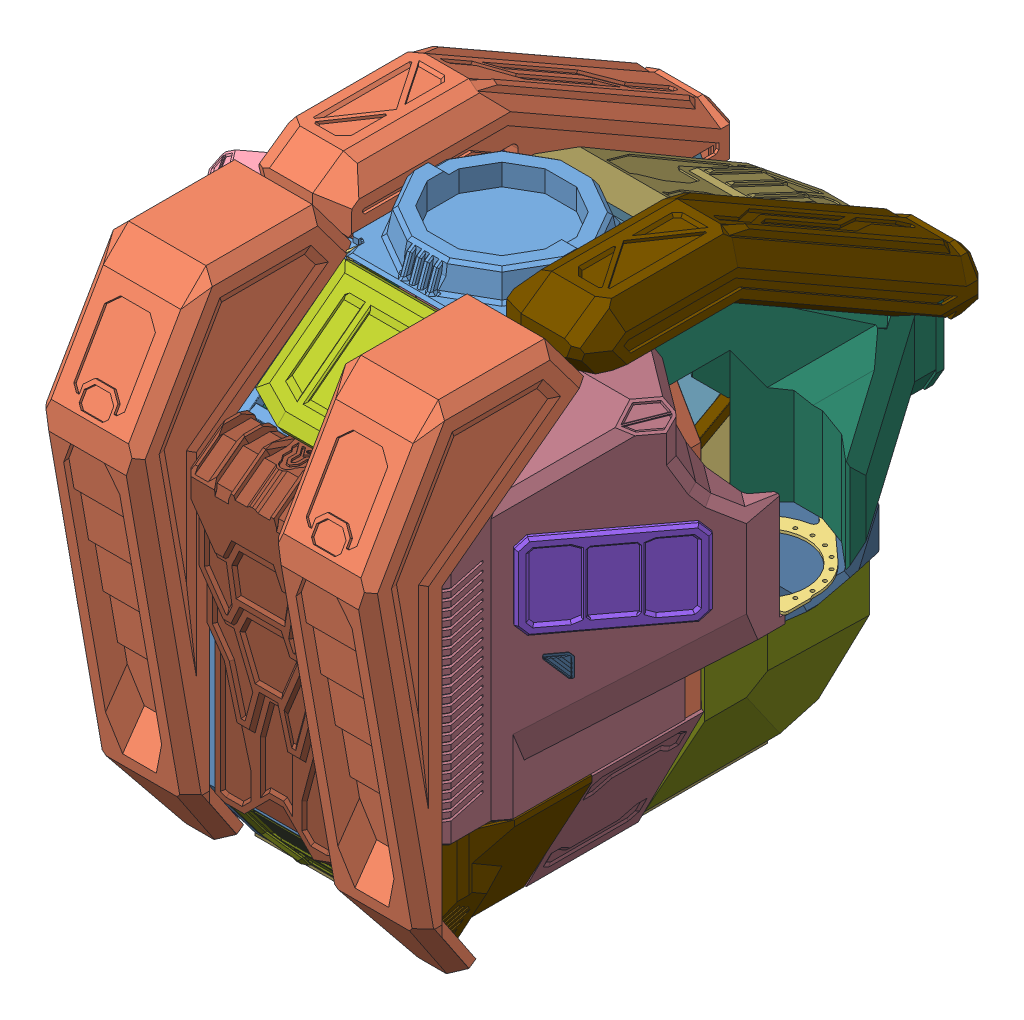
SolidWorks assembly cockpite superficie, configuration Défaut. Lengths in mm.
Overall size (2088.81 2085.24 2703.64).
117 component instances, 75 part files, 251 mates.
Components (placement in the parent):
- cockpit_segmentLAT_0-1: cockpit_segmentLAT_0 [Défaut] at origin size (80 1780 1700)
- cockpit_segmentLAT_0-2: cockpit_segmentLAT_0 [Défaut] at (-580 0 0) size (80 1780 1700)
- cockpit_segmentFACE_0-1: cockpit_segmentFACE_0 [Défaut] at (-250 0 -10.6226) size (1180 1780 80)
- Manikin_sit-1: Manikin_sit [Default] at (-178.4008 -3076.5165 -521.6706) x (-0.998263 -0.006408 -0.058563) z (0.055728 0.219684 -0.973978) size (878.99 1461.66 750.53)
  - Hips-1: Hips [Default] at (41.9716 15.4252 492.0452) x (0.998799 0.006411 -0.048571) z (0.047333 0.129538 0.990444) size (295.24 313.39 270.97)
  - Torso-1: Torso [Default] at (-29.1895 18.5281 -268.9557) x (0.995716 0.002037 -0.092438) z (0.092349 -0.071067 0.993187) size (460.89 555.97 263.41)
  - Head-2: Head [Default] at (-35.3994 3.8201 -64.7195) x (0.99996 -0.00842 0.002952) z (-0.003142 -0.022585 0.99974) size (157.49 285.21 225.45)
  - ArmLeftUpper-1: ArmLeftUpper [Default] at (-1722.5354 534.7955 -622.021) x (0.903661 -0.428241 0.002425) z (-0.067425 -0.136682 0.988318) size (245.85 241.52 164.39)
  - LegLeftUpper-1: LegLeftUpper [Default] at (-298.9777 2948.9846 3668.472) x (0.995737 -0.057217 0.072354) z (0.044237 0.984495 0.169742) size (217.98 507.99 239.38)
  - ArmLeftFore-1: ArmLeftFore [Default] at (-2325.1537 1043.3966 992.7578) x (0.576966 -0.135199 0.8055) z (-0.537701 0.679474 0.499192) size (231.54 177.84 142.38)
  - ArmLeftHand-1: ArmLeftHand [Default] at (-1973.6621 823.2165 1249.8034) x (0.681315 -0.092916 0.72607) z (-0.527105 0.625983 0.574722) size (149.66 182.81 147.58)
  - LegLeftLower-1: LegLeftLower [Default] at (-393.4208 426.2264 1183.139) x (0.993791 -0.108531 0.024512) z (0.002157 0.239057 0.971003) size (171.81 443.68 193.78)
  - LegLeftFoot-1: LegLeftFoot [Default] at (-391.5322 345.3545 592.5292) x (0.993832 -0.110241 0.012061) z (-0.008622 0.031619 0.999463) size (154.71 147.12 252.53)
  - ArmRightUpper-1: ArmRightUpper [Default] at (2412.2824 931.5079 323.6395) x (0.78978 0.59507 0.148794) z (-0.156135 -0.039556 0.986943) size (246.03 241.06 163.63)
  - ArmRightFore-1: ArmRightFore [Default] at (2450.4069 1513.5578 1822.4726) x (0.754277 0.265812 -0.600342) z (0.232424 0.747064 0.622796) size (231.51 177.54 142.76)
  - ArmRightHand-1: ArmRightHand [Default] at (726.3463 519.61 2107.5247) x (0.731421 -0.279768 -0.621895) z (0.656431 0.535891 0.530961) size (149.56 182.72 147.2)
  - LegRightUpper-1: LegRightUpper [Default] at (121.5915 3105.6896 3713.3645) x (0.987695 0.156074 -0.009999) z (-0.153555 0.97991 0.127269) size (216.84 507.94 244.77)
  - LegRightLower-1: LegRightLower [Default] at (672.1591 446.131 902.2036) x (0.976643 0.210274 0.044195) z (-0.073882 0.135492 0.98802) size (171.15 451.19 193.59)
  - LegRightFoot-1: LegRightFoot [Default] at (695.8533 419.9505 536.4877) x (0.976144 0.210831 0.051905) z (-0.054843 0.008108 0.998462) size (155.81 152.18 252.53)
- cockpit_segment_40x40_0-1: cockpit_segment_40x40_0 [Défaut] at (80 1283.2129 -10) size (258 40 730)
- cockpit_segment_40x40_0-2: cockpit_segment_40x40_0 [Défaut] at (-580 1323.2129 -10) x (-1 0 0) z (0 0 1) size (258 40 730)
- cockpit_segment_40x40_0-3: cockpit_segment_40x40_0 [Défaut] at (80 960 -10) size (258 40 730)
- cockpit_segment_40x40_0-4: cockpit_segment_40x40_0 [Défaut] at (-580 1000 -10) x (-1 0 0) z (0 0 1) size (258 40 730)
- cockpit_segmentFACE_0-2: cockpit_segmentFACE_0 [Défaut] at (-250 0 333.3333) size (1180 1780 80)
- cockpit_poutre40x80x500-5: cockpit_poutre40x80x500 [Défaut] at (-500 250 920) x (0 1 0) z (1 0 0) size (80 40 500)
- cockpit_poutre40x80x500-6: cockpit_poutre40x80x500 [Défaut] at (0 1330 920) x (0 -1 0) z (-1 0 0) size (80 40 500)
- cockpit_poutre40x80x500-7: cockpit_poutre40x80x500 [Défaut] at (-500 -40 -436.5685) x (0 0 -1) z (1 0 0) size (80 40 500)
- cockpit_poutre40x40x366-1: cockpit_poutre40x40x366 [Défaut] at (-840 1270.6802 69.3333) size (40 40 264)
- cockpit_poutre40x40x366-2: cockpit_poutre40x40x366 [Défaut] at (-840 440.3702 69.3333) size (40 40 264)
- cockpit_poutre40x40x366-3: cockpit_poutre40x40x366 [Défaut] at (300 1270.6802 69.3774) size (40 40 264)
- cockpit_poutre40x40x366-4: cockpit_poutre40x40x366 [Défaut] at (300 440.3702 69.3774) size (40 40 264)
- cockpit_poutre40x40x366-5: cockpit_poutre40x40x366 [Défaut] at (-840 960 67.3333) size (40 40 264)
- cockpit_poutre40x40x366-6: cockpit_poutre40x40x366 [Défaut] at (300 960 69.3774) size (40 40 264)
- bras_fixation_1-1: bras_fixation_1 [Défaut] at (340 990 512.9113) size (615.49 10 1037.05)
- bras_fixation_1-2: bras_fixation_1 [Défaut] at (-840 1000 512.9113) x (-1 0 0) z (0 0 1) size (615.49 10 1037.05)
- cockpit_poutre40x80x500-8: cockpit_poutre40x80x500 [Défaut] at (-500 396.2581 380) x (0 1 0) z (1 0 0) size (80 40 500)
- traverse_pente1-1: traverse_pente1 [Défaut] at (338 209.1038 -10.6226) x (-1 0 0) z (0 0 -1) size (257.78 292.58 728.37)
- traverse_pente1_sym-1: traverse_pente1_sym [Défaut] at (-838 209.1038 -10.6226) size (257.78 292.58 733.7)
- cockpit_poutre40x80x500-9: cockpit_poutre40x80x500 [Défaut] at (0 1340.3258 816.6212) x (0 0.90883 0.417168) z (-1 0 0) size (80 40 500)
- cockpit_segment_40x40_1_soutien_bras-1: cockpit_segment_40x40_1_soutien_bras [Défaut] at (-840 990 69.3774) x (0 -1 0) z (1 0 0) size (350 80 400)
- cockpit_segment_40x40_1_soutien_bras-2: cockpit_segment_40x40_1_soutien_bras [Défaut] at (340 990 -10.6226) x (0 -1 0) z (-1 0 0) size (350 80 400)
- cockpit_segment_40x40_2_back-1: cockpit_segment_40x40_2_back [Défaut] at (80 1310.6802 413.3333) x (1 0 0) z (0 0 -1) size (260 40 546)
- cockpit_segment_40x40_2_back-2: cockpit_segment_40x40_2_back [Défaut] at (-580 1270.6802 413.3333) x (-1 0 0) z (0 0 -1) size (260 40 546)
- attache_porte-1: attache_porte [Défaut] at (-500 1641.4369 -183.108) x (0 0.496139 0.868243) z (-1 0 0) size (198.66 73.18 10)
- attache_porte-2: attache_porte [Défaut] at (80 1641.4369 -183.108) x (0 0.496139 0.868243) z (-1 0 0) size (198.66 73.18 10)
- attache_porte-3: attache_porte [Défaut] at (-570 1641.4369 -183.108) x (0 0.496139 0.868243) z (-1 0 0) size (198.66 73.18 10)
- attache_porte-4: attache_porte [Défaut] at (10 1641.4369 -183.108) x (0 0.496139 0.868243) z (-1 0 0) size (198.66 73.18 10)
- axeO20.25_700-1: axeO20.25_700 [Défaut] at (-600 1702.1061 -146.8375) x (0 0.072457 -0.997372) z (1 0 0) size (20 20 700)
- Capot-1: Capot [Défaut] at (-480 1702.1061 -146.8375) x (-1 0 0) z (0 -0.505329 -0.862927) size (560 946.97 1454.08)
  - Capot1-1: Capot1 [Défaut] at origin size (10 749.16 1208.3)
  - Capot1-2: Capot1 [Défaut] at (-470 0 0) size (10 749.16 1208.3)
  - cockpit_poutre40x40x480-1: cockpit_poutre40x40x480 [Défaut] at (10 -20 40) x (0 0 1) z (-1 0 0) size (40 40 480)
  - cockpit_poutre40x40x480-2: cockpit_poutre40x40x480 [Défaut] at (10 -32.3205 751.7543) x (0 0.866025 0.5) z (-1 0 0) size (40 40 480)
  - cockpit_poutre40x40x480-3: cockpit_poutre40x40x480 [Défaut] at (10 -683.1793 1118.6603) x (0 -0.866025 0.5) z (-1 0 0) size (40 40 480)
  - Capot2-1: Capot2 [Défaut] at (-230 -26.9447 40) x (-1 0 0) z (0 0 -1) size (560 161.69 1100)
  - Capot3-1: Capot3 [Défaut] at (20 -892.9701 1297.518) x (-1 0 0) z (0 -0.5 -0.866025) size (500 906.77 276.51)
  - Capot4-1: Capot4 [Défaut] at (-470 0 0) x (0 0 -1) z (1 0 0) size (133 66 480)
- deco_torse1-1: deco_torse1 [Défaut] at (277.9178 1000 -180) size (738.18 710 1099)
- deco_torse2RIGHT-1: deco_torse2RIGHT [Défaut] at (336.2329 150 -15) size (343.72 998.15 825)
- deco_torse2LEFT-1: deco_torse2LEFT [Défaut] at (-173.0822 150 -15) size (343.72 998.15 825)
- deco_torse3_upRIGHT-1: deco_torse3_upRIGHT [Défaut] at (40.1918 1340 -57.5) x (0 0 -1) z (1 0 0) size (1491.8 695.65 350)
- deco_headcollar-1: deco_headcollar [Défaut] at (-540 1740 423.19) size (580 120 645)
- deco_torse4_back-1: deco_torse4_back [Défaut] at (0 250 960) size (370 1970 842.42)
  - deco_torse4_back-1: deco_torse4_back [Défaut] at origin size (370 1970 842.42)
- deco_torse4_back-2: deco_torse4_back [Défaut] at (-870 250 960) size (370 1970 842.42)
  - deco_torse4_back-1: deco_torse4_back [Défaut] at origin size (370 1970 842.42)
- attache_porte2-2: attache_porte2 [Défaut] at (0 1653 529.3333) x (0 0.6 -0.8) z (1 0 0) size (145 61.12 10)
- attache_porte2-4: attache_porte2 [Défaut] at (-510 1653 529.3333) x (0 0.6 -0.8) z (1 0 0) size (145 61.12 10)
- deco_torse5_back-1: deco_torse5_back [Défaut] at (-674.9206 1000 214) x (-1 0 0) z (0 0 -1) size (654 1290 891)
- deco_torse1_sym-1: deco_torse1_sym [Défaut] at (-238.4658 1000 -180) size (738.18 710 1099)
- axeO20_520-1: axeO20_520 [Défaut] at (10 1717.0991 489.9076) x (0 0 1) z (-1 0 0) size (20 20 520)
- écoutille1-1: écoutille1 [Défaut] at (-495 1713.4141 461.8644) x (0 -0.608956 0.793204) z (-1 0 0) size (485 60 490)
- back_trap-1: back_trap [Défaut] at (-1165.1221 1068.7153 290.3244) x (0.600343 0 0.799743) z (-0.799743 0 0.600343) size (530 320 30)
- deco_torse6_airvent-1: deco_torse6_airvent [Défaut] at (-834.9206 990 -10.6226) x (0 -1 0) z (1 0 0) size (382 611.74 504.34)
- airvent-1: airvent [Défaut] at (-958.7971 986.7153 581.836) x (0 -1 0) z (-0.600343 0 -0.799743) size (85 14 85)
- deco_torse7_dos-1: deco_torse7_dos [Défaut] at (0 230 960) x (-1 0 0) z (0 0 -1) size (500 1212.5 230)
- plancher-1: plancher [Défaut] at (-580 -50 740.5405) size (660 10 1260)
- deco_torse8_lateralinferieur-1: deco_torse8_lateralinferieur [Défaut] at (-599.1619 -30.8347 -6.6667) x (0 0 1) z (-0.890435 -0.455111 0) size (420 540 10)
- deco_torse8_lateralinferieur-2: deco_torse8_lateralinferieur [Défaut] at (99.1619 -30.8347 413.3333) x (0 0 -1) z (0.890435 -0.455111 0) size (420 540 10)
- attache_porte-5: attache_porte [Défaut] at (0 100.474 -657.0426) x (0 -0.707107 0.707107) z (1 0 0) size (198.66 73.18 10)
- attache_porte-6: attache_porte [Défaut] at (-510 100.474 -657.0426) x (0 -0.707107 0.707107) z (1 0 0) size (198.66 73.18 10)
- axeO20_520-2: axeO20_520 [Défaut] at (10 32.3991 -638.0132) x (0 0 1) z (-1 0 0) size (20 20 520)
- internalpanel1_back-1: internalpanel1_back [Défaut] at (-580 1402.9178 801.3393) x (1 0 0) z (0 0.417168 -0.90883) size (660 1010 10)
- internalpanel2_side-1: internalpanel2_side [Défaut] at (300 450 -10.6226) x (0 0 1) z (-1 0 0) size (424 850 10)
- internalpanel2_side-2: internalpanel2_side [Défaut] at (-800 450 413.3774) x (0 0 -1) z (1 0 0) size (424 850 10)
- internalpanel3_upside-1: internalpanel3_upside [Défaut] at (-799.2967 1301.2231 413.3774) x (0 0 -1) z (0.866906 -0.498471 0) size (424 460 10)
- internalpanel3_upside-2: internalpanel3_upside [Défaut] at (299.2967 1301.2231 -10.6226) x (0 0 1) z (-0.866906 -0.498471 0) size (424 460 10)
- internalpanel4_downside-1: internalpanel4_downside [Défaut] at (70 0 -10.6226) x (0 0 1) z (-0.890435 0.455111 0) size (424 503 10)
- internalpanel4_downside-2: internalpanel4_downside [Défaut] at (-570 0 413.3333) x (0 0 -1) z (0.890435 0.455111 0) size (424 503 10)
- internalpanel5_downback-1: internalpanel5_downback [Défaut] at (80 0 380) x (-1 0 0) z (0 0 -1) size (660 485 10)
- internalpanel6_floor-1: internalpanel6_floor [Défaut] at (80 0 -500) x (-1 0 0) z (0 1 0) size (660 870 10)
- sparco style race seat 1-1: sparco style race seat 1 [Default] at (-243.2192 277.46 345.725) x (0 0 1) z (-1 0 0) size (757.44 888.09 564.73)
- internalpanel7_frontLEFT-2: internalpanel7_frontLEFT [Défaut] at (13.6774 450 -703.8176) x (0.381763 0 0.92426) z (-0.92426 0 0.381763) size (750 1100 10)
- internalpanel8_frontRIGHT-1: internalpanel8_frontRIGHT [Défaut] at (-1086.3226 450 682.5725) x (0.381763 0 -0.92426) z (0.92426 0 0.381763) size (750 1100 10)
- internalpanel9_frontLup-1: internalpanel9_frontLup [Défaut] at (288.8206 1299.3811 -10.6226) x (-0.291598 -0.167669 -0.941731) z (0.816393 0.469426 -0.336366) size (736.22 460 3)
- internalpanel9_frontLup-2: internalpanel9_frontLup [Défaut] at (-791.2698 1300.7894 -11.6317) x (0.291598 -0.167669 -0.941731) z (0.816393 -0.469426 0.336366) size (736.22 460 3)
- internalpanel10_backsideLEFT-1: internalpanel10_backsideLEFT [Défaut] at (-580 485 380) x (0 0 -1) z (1 0 0) size (374.1 815 210)
- internalpanel10.5_backsideLEFT-1: internalpanel10.5_backsideLEFT [Défaut] at (-580 485 380) x (-1 0 0) z (0 0 -1) size (210 1220 10)
- internalpanel10_backsideRIGHT-1: internalpanel10_backsideRIGHT [Défaut] at (500 485 388.3406) x (0 0 -1) z (1 0 0) size (374.1 815 210)
- internalpanel10.5_backsideRIGHT-1: internalpanel10.5_backsideRIGHT [Défaut] at (80 485 388.3406) x (-1 0 0) z (0 0 -1) size (210 1220 10)
- deco_torse6_airventRIGHT-1: deco_torse6_airventRIGHT [Défaut] at (-281.076 990 -304.901) x (0 -1 0) z (0.628361 0 0.777922) size (382 438.89 781.29)
- internalpanel11_backsideUPLEFT-1: internalpanel11_backsideUPLEFT [Défaut] at (-800 1310.6802 413.3774) x (0 0 -1) z (1 0 0) size (385 365.22 210)
- internalpanel11_backsideUPRIGHT-1: internalpanel11_backsideUPRIGHT [Défaut] at (-140 1312.1 413.3333) x (0 0 -1) z (1 0 0) size (385 365.22 210)
- deco_torse5_backRIGHT-1: deco_torse5_backRIGHT [Défaut] at (1294 1000 214) x (-1 0 0) z (0 0 -1) size (654 1290 891)
- airvent-2: airvent [Défaut] at (457.8765 986.7153 581.836) x (-0.600343 0 0.799743) z (0 1 0) size (85 14 85)
- back_trap-2: back_trap [Défaut] at (358.0266 1068.7153 698.1932) x (0.600343 0 -0.799743) z (0.799743 0 0.600343) size (530 320 30)
- front_trapLEFT-1: front_trapLEFT [Défaut] at (-238.4658 1000 -910) x (-1 0 0) z (0 0 -1) size (311.73 350 50)
- front_trapRIGHT-1: front_trapRIGHT [Défaut] at (277.9178 1000 -910) x (-1 0 0) z (0 0 -1) size (311.73 350 50)
- deco_torse9_backbas-1: deco_torse9_backbas [Défaut] at (-500 -41.7099 725.6986) x (1 0 0) z (0 -0.603443 0.797406) size (500 371.41 25)
- deco_torse10_backbassideLEFT-1: deco_torse10_backbassideLEFT [Défaut] at (-855 -40 413.3333) size (275 490 530)
- deco_torse10_backbassideRIGHT-1: deco_torse10_backbassideRIGHT [Défaut] at (-195 -40 413.3333) size (275 490 530)
- écoutille2-1: écoutille2 [Défaut] at (0 -20.8559 -595.7178) x (-1 0 0) z (0 -0.36413 -0.931348) size (500 589.73 150)
- deco_torse3_upLEFT-1: deco_torse3_upLEFT [Défaut] at (-540.1918 1340 -57.5) x (0 0 -1) z (1 0 0) size (1491.8 695.65 350)
- attache_verin_cokpitepaul-1: attache_verin_cokpitepaul [Défaut] at (-739.6995 1260.6802 553.842) x (0.707107 0 -0.707107) z (0 1 0) size (92.03 103.34 10)
- attache_verin_cokpitepaul-2: attache_verin_cokpitepaul [Défaut] at (-739.6995 1190.6802 553.842) x (0.707107 0 -0.707107) z (0 1 0) size (92.03 103.34 10)
- attache_verin_cokpitepaul-3: attache_verin_cokpitepaul [Défaut] at (239.6995 1270.6802 553.842) x (-0.707107 0 -0.707107) z (0 -1 0) size (92.03 103.34 10)
- attache_verin_cokpitepaul-4: attache_verin_cokpitepaul [Défaut] at (119.4914 1190.6802 433.6338) x (0.707107 0 0.707107) z (0 1 0) size (92.03 103.34 10)
Mates (geometry in assembly coordinates):
- Distance1: distance = 500 mm anti-aligned: plane of cockpit_segmentLAT_0-1 through (0 0 0) normal (-1 0 0); plane of cockpit_segmentLAT_0-2 through (-500 0 0) normal (1 0 0)
- Coïncidente2: coincident aligned: plane of cockpit_segmentLAT_0-1 through (80 0 -740) normal (0 0 -1); plane of cockpit_segmentLAT_0-2 through (-500 0 -740) normal (0 0 -1)
- Coïncidente3: coincident aligned: plane of cockpit_segmentLAT_0-2 through (-500 1740 0) normal (0 1 0); plane of cockpit_segmentLAT_0-1 through (80 1740 0) normal (0 1 0)
- Coïncidente4: coincident aligned: plane of cockpit_segmentLAT_0-2 through (-500 1740 0) normal (0 1 0); plane of cockpit_segmentFACE_0-1 through (-593.1411 1740 69.3774) normal (0 1 0)
- Coïncidente5: coincident: line of cockpit_segmentLAT_0-1 through (78 1740 -10.6226) axis (-1 0 0); plane of cockpit_segmentFACE_0-1 through (-250 0 -10.6226) normal (0 0 -1)
- Distance2: distance = 250 mm: point of cockpit_segmentFACE_0-1; plane of cockpit_segmentLAT_0-2 through (-500 0 0) normal (1 0 0)
- Coïncidente7: coincident anti-aligned: plane of cockpit_segmentLAT_0-1 through (80 0 0) normal (1 0 0); plane of cockpit_segment_40x40_0-1 through (80 1323.2129 -619.9611) normal (-1 0 0)
- Coïncidente8: coincident: plane of cockpit_segmentLAT_0-1 through (80 0 -740) normal (0 0 -1); line of cockpit_segment_40x40_0-1 through (80 1321.2129 -740) axis (0 -1 0)
- Coïncidente9: coincident: line of cockpit_segmentLAT_0-1 through (78 1323.2129 -740) axis (-1 0 0); plane of cockpit_segment_40x40_0-1 through (80 1323.2129 -10) normal (0 1 0)
- Coïncidente11: coincident anti-aligned: plane of cockpit_segmentLAT_0-2 through (-580 0 0) normal (-1 0 0); plane of cockpit_segment_40x40_0-2 through (-580 1283.2129 -619.9611) normal (1 0 0)
- Coïncidente14: coincident: line of cockpit_segmentLAT_0-2 through (-502 1323.2129 -740) axis (-1 0 0); plane of cockpit_segment_40x40_0-2 through (-580 1323.2129 -10) normal (0 1 0)
- Coïncidente15: coincident: plane of cockpit_segmentLAT_0-2 through (-500 0 -740) normal (0 0 -1); line of cockpit_segment_40x40_0-2 through (-580 1285.2129 -740) axis (0 1 0)
- Coïncidente16: coincident anti-aligned: plane of cockpit_segmentLAT_0-1 through (80 0 0) normal (1 0 0); plane of cockpit_segment_40x40_0-3 through (80 1000 -619.9611) normal (-1 0 0)
- Coïncidente17: coincident: plane of cockpit_segmentLAT_0-1 through (80 0 -740) normal (0 0 -1); line of cockpit_segment_40x40_0-3 through (80 998 -740) axis (0 -1 0)
- Coïncidente18: coincident anti-aligned: plane of cockpit_segmentLAT_0-2 through (-580 0 0) normal (-1 0 0); plane of cockpit_segment_40x40_0-4 through (-580 960 -619.9611) normal (1 0 0)
- Coïncidente19: coincident: plane of cockpit_segmentLAT_0-2 through (-500 0 -740) normal (0 0 -1); line of cockpit_segment_40x40_0-4 through (-580 962 -740) axis (0 1 0)
- Coïncidente20: coincident aligned: plane of cockpit_segment_40x40_0-3 through (80 960 -10) normal (0 -1 0); plane of cockpit_segment_40x40_0-4 through (-580 960 -10) normal (0 -1 0)
- Coïncidente21: coincident aligned: plane of cockpit_segmentFACE_0-1 through (-593.1411 1740 69.3774) normal (0 1 0); plane of cockpit_segmentFACE_0-2 through (-593.1411 1740 413.3333) normal (0 1 0)
- Coïncidente22: coincident aligned: plane of cockpit_segmentFACE_0-1 through (-840 1310.6802 69.3774) normal (-1 0 0); plane of cockpit_segmentFACE_0-2 through (-840 1310.6802 413.3333) normal (-1 0 0)
- Coïncidente23: coincident: line of cockpit_segmentLAT_0-1 through (78 1740 413.3333) axis (-1 0 0); plane of cockpit_segmentFACE_0-2 through (-250 0 413.3333) normal (0 0 1)
- Coïncidente25: coincident aligned: plane of cockpit_segmentLAT_0-2 through (-500 -40 0) normal (0 -1 0); plane of cockpit_poutre40x80x500-7 through (0 -40 -438.5685) normal (0 -1 0)
- Coïncidente26: coincident anti-aligned: plane of cockpit_segmentLAT_0-2 through (-500 0 0) normal (1 0 0); plane of cockpit_poutre40x80x500-7 through (-500 -38 -438.5685) normal (-1 0 0)
- Coïncidente27: coincident: line of cockpit_segmentLAT_0-2 through (-502 -40 -516.5685) axis (-1 0 0); plane of cockpit_poutre40x80x500-7 through (0 -38 -516.5685) normal (0 0 -1)
- Coïncidente35: coincident aligned: plane of cockpit_segmentFACE_0-1 through (-840 1310.6802 69.3774) normal (-1 0 0); plane of cockpit_poutre40x40x366-1 through (-840 1272.6802 333.3333) normal (-1 0 0)
- Coïncidente36: coincident aligned: plane of cockpit_segmentFACE_0-1 through (-840 1310.6802 69.3774) normal (-1 0 0); plane of cockpit_poutre40x40x366-2 through (-840 442.3702 333.3333) normal (-1 0 0)
- Coïncidente37: coincident: line of cockpit_segmentFACE_0-1 through (-840 1310.6802 67.3774) axis (0 0 -1); plane of cockpit_poutre40x40x366-1 through (-838 1310.6802 333.3333) normal (0 1 0)
- Coïncidente38: coincident: line of cockpit_segmentFACE_0-1 through (-840 440.3702 67.3774) axis (0 0 -1); plane of cockpit_poutre40x40x366-2 through (-838 440.3702 333.3333) normal (0 -1 0)
- Coïncidente39: coincident anti-aligned: plane of cockpit_segmentFACE_0-2 through (-250 0 333.3333) normal (0 0 -1); plane of cockpit_poutre40x40x366-1 through (-838 1272.6802 333.3333) normal (0 0 1)
- Coïncidente40: coincident anti-aligned: plane of cockpit_segmentFACE_0-2 through (-250 0 333.3333) normal (0 0 -1); plane of cockpit_poutre40x40x366-2 through (-838 442.3702 333.3333) normal (0 0 1)
- Coïncidente41: coincident aligned: plane of cockpit_segmentFACE_0-2 through (340 1310.6802 413.3333) normal (1 0 0); plane of cockpit_poutre40x40x366-3 through (340 1272.6802 333.3774) normal (1 0 0)
- Coïncidente42: coincident: line of cockpit_segmentFACE_0-2 through (340 1310.6802 411.3333) axis (0 0 -1); plane of cockpit_poutre40x40x366-3 through (302 1310.6802 333.3774) normal (0 1 0)
- Coïncidente43: coincident anti-aligned: plane of cockpit_segmentFACE_0-1 through (-250 0 69.3774) normal (0 0 1); plane of cockpit_poutre40x40x366-3 through (302 1272.6802 69.3774) normal (0 0 -1)
- Coïncidente44: coincident aligned: plane of cockpit_segmentFACE_0-2 through (340 1310.6802 413.3333) normal (1 0 0); plane of cockpit_poutre40x40x366-4 through (340 442.3702 333.3774) normal (1 0 0)
- Coïncidente45: coincident: line of cockpit_segmentFACE_0-2 through (340 440.3702 411.3333) axis (0 0 -1); plane of cockpit_poutre40x40x366-4 through (302 440.3702 333.3774) normal (0 -1 0)
- Coïncidente47: coincident anti-aligned: plane of cockpit_segmentFACE_0-1 through (-250 0 69.3774) normal (0 0 1); plane of cockpit_poutre40x40x366-4 through (302 442.3702 69.3774) normal (0 0 -1)
- Distance3: distance = 1000 mm aligned: plane of cockpit_segment_40x40_0-3 through (80 960 -10) normal (0 -1 0); plane of cockpit_segmentLAT_0-1 through (80 -40 0) normal (0 -1 0)
- Coïncidente49: coincident aligned: plane of cockpit_segment_40x40_0-3 through (80 1000 -10) normal (0 1 0); plane of cockpit_poutre40x40x366-6 through (302 1000 333.3774) normal (0 1 0)
- Coïncidente50: coincident aligned: plane of cockpit_segment_40x40_0-4 through (-580 1000 -10) normal (0 1 0); plane of cockpit_poutre40x40x366-5 through (-838 1000 331.3333) normal (0 1 0)
- Coïncidente51: coincident aligned: plane of cockpit_segmentFACE_0-1 through (340 1310.6802 69.3774) normal (1 0 0); plane of cockpit_poutre40x40x366-6 through (340 962 333.3774) normal (1 0 0)
- Coïncidente52: coincident anti-aligned: plane of cockpit_segmentFACE_0-1 through (-250 0 69.3774) normal (0 0 1); plane of cockpit_poutre40x40x366-6 through (302 962 69.3774) normal (0 0 -1)
- Coïncidente53: coincident aligned: plane of cockpit_segmentFACE_0-1 through (-840 1310.6802 69.3774) normal (-1 0 0); plane of cockpit_poutre40x40x366-5 through (-840 962 331.3333) normal (-1 0 0)
- Coïncidente61: coincident aligned: plane of cockpit_segment_40x40_0-3 through (80 1000 -10) normal (0 1 0); plane of bras_fixation_1-1 through (540 1000 -47.0887) normal (0 1 0)
- Coïncidente63: coincident aligned: plane of cockpit_segment_40x40_0-4 through (-580 1000 -10) normal (0 1 0); plane of bras_fixation_1-2 through (-1040 1000 -47.0887) normal (0 1 0)
- Coïncidente70: coincident aligned: line of cockpit_segmentLAT_0-1 through (78 1330 960) axis (-1 0 0); plane of cockpit_poutre40x80x500-6 through (-500 1330 922) normal (0 1 0)
- Coïncidente71: coincident anti-aligned: plane of cockpit_segmentLAT_0-1 through (0 0 0) normal (-1 0 0); plane of cockpit_poutre40x80x500-6 through (0 1328 922) normal (1 0 0)
- Coïncidente72: coincident aligned: plane of cockpit_segmentLAT_0-1 through (80 0 960) normal (0 0 1); plane of cockpit_poutre40x80x500-6 through (-500 1328 960) normal (0 0 1)
- Coïncidente73: coincident aligned: plane of cockpit_segmentLAT_0-2 through (-500 0 960) normal (0 0 1); plane of cockpit_poutre40x80x500-5 through (0 252 960) normal (0 0 1)
- Coïncidente74: coincident anti-aligned: plane of cockpit_segmentLAT_0-2 through (-500 0 0) normal (1 0 0); plane of cockpit_poutre40x80x500-5 through (-500 252 922) normal (-1 0 0)
- Coïncidente75: coincident: line of cockpit_segmentLAT_0-1 through (78 250 960) axis (-1 0 0); plane of cockpit_poutre40x80x500-5 through (0 250 922) normal (0 -1 0)
- Coïncidente76: coincident aligned: plane of cockpit_segmentLAT_0-1 through (80 0 420) normal (0 0 1); plane of cockpit_poutre40x80x500-8 through (0 398.2581 420) normal (0 0 1)
- Coïncidente77: coincident anti-aligned: plane of cockpit_segmentLAT_0-2 through (-500 0 0) normal (1 0 0); plane of cockpit_poutre40x80x500-8 through (-500 398.2581 382) normal (-1 0 0)
- Coïncidente78: coincident: line of cockpit_segmentLAT_0-2 through (-502 476.2581 420) axis (-1 0 0); plane of cockpit_poutre40x80x500-8 through (0 476.2581 382) normal (0 1 0)
- Coïncidente83: coincident anti-aligned: plane of cockpit_segmentLAT_0-1 through (80 0 0) normal (1 0 0); plane of traverse_pente1-1 through (80 469.3117 -739.6226) normal (-1 0 0)
- Coïncidente86: coincident anti-aligned: plane of cockpit_segmentFACE_0-1 through (-250 0 -10.6226) normal (0 0 -1); plane of traverse_pente1-1 through (338 209.1038 -10.6226) normal (0 0 1)
- Coïncidente92: coincident: line of cockpit_segmentLAT_0-1 through (80 -38 -515.7401) axis (0 0.707107 -0.707107); point of traverse_pente1-1
- Coïncidente93: coincident anti-aligned: plane of cockpit_segmentFACE_0-1 through (-250 0 -10.6226) normal (0 0 -1); plane of traverse_pente1_sym-1 through (-835.8915 172.5363 -10.6226) normal (0 0 1)
- Coïncidente96: coincident anti-aligned: plane of cockpit_segmentLAT_0-2 through (-580 0 0) normal (-1 0 0); plane of traverse_pente1_sym-1 through (-580 469.3117 -739.6226) normal (1 0 0)
- Coïncidente98: coincident: line of cockpit_segmentLAT_0-2 through (-580 184.2599 -738) axis (0 -0.707107 0.707107); point of traverse_pente1_sym-1
- Coïncidente102: coincident aligned: plane of cockpit_segmentLAT_0-2 through (-500 -76.3537 166.3421) normal (0 -0.417168 0.90883); plane of cockpit_poutre40x80x500-9 through (-500 1342.1434 817.4555) normal (0 -0.417168 0.90883)
- Coïncidente103: coincident anti-aligned: plane of cockpit_segmentLAT_0-2 through (-500 0 0) normal (1 0 0); plane of cockpit_poutre40x80x500-9 through (-500 1342.9778 815.6379) normal (-1 0 0)
- Coïncidente108: coincident anti-aligned: plane of cockpit_segmentFACE_0-1 through (340 1310.6802 69.3774) normal (1 0 0); plane of cockpit_segment_40x40_1_soutien_bras-2 through (340 693.1507 69.3774) normal (-1 0 0)
- Coïncidente109: coincident anti-aligned: plane of bras_fixation_1-1 through (540 990 -47.0887) normal (0 -1 0); plane of cockpit_segment_40x40_1_soutien_bras-2 through (679.2563 990 69.3774) normal (0 1 0)
- Coïncidente110: coincident aligned: plane of cockpit_segmentFACE_0-1 through (-250 0 -10.6226) normal (0 0 -1); plane of cockpit_segment_40x40_1_soutien_bras-2 through (340 990 -10.6226) normal (0 0 -1)
- Coïncidente114: coincident anti-aligned: plane of cockpit_segmentFACE_0-2 through (-840 1310.6802 413.3333) normal (-1 0 0); plane of cockpit_segment_40x40_1_soutien_bras-1 through (-840 693.1507 -10.6226) normal (1 0 0)
- Coïncidente115: coincident anti-aligned: plane of bras_fixation_1-2 through (-1040 990 -47.0887) normal (0 -1 0); plane of cockpit_segment_40x40_1_soutien_bras-1 through (-1179.2563 990 -10.6226) normal (0 1 0)
- Coïncidente116: coincident aligned: plane of cockpit_segmentFACE_0-1 through (-250 0 -10.6226) normal (0 0 -1); plane of cockpit_segment_40x40_1_soutien_bras-1 through (-840 990 -10.6226) normal (0 0 -1)
- Coïncidente117: coincident anti-aligned: plane of cockpit_segmentFACE_0-2 through (-250 0 413.3333) normal (0 0 1); plane of cockpit_segment_40x40_2_back-2 through (-795.6964 1310.6802 413.3333) normal (0 0 -1)
- Coïncidente118: coincident anti-aligned: plane of cockpit_segmentLAT_0-2 through (-580 0 0) normal (-1 0 0); plane of cockpit_segment_40x40_2_back-2 through (-580 1310.6802 866.2957) normal (1 0 0)
- Coïncidente119: coincident aligned: plane of cockpit_poutre40x40x366-1 through (-838 1310.6802 333.3333) normal (0 1 0); plane of cockpit_segment_40x40_2_back-2 through (-580 1310.6802 413.3333) normal (0 1 0)
- Coïncidente121: coincident anti-aligned: plane of cockpit_segmentFACE_0-2 through (-250 0 413.3333) normal (0 0 1); plane of cockpit_segment_40x40_2_back-1 through (295.6964 1270.6802 413.3333) normal (0 0 -1)
- Coïncidente122: coincident anti-aligned: plane of cockpit_segmentLAT_0-1 through (80 0 0) normal (1 0 0); plane of cockpit_segment_40x40_2_back-1 through (80 1270.6802 866.2957) normal (-1 0 0)
- Coïncidente123: coincident aligned: plane of cockpit_poutre40x40x366-3 through (302 1310.6802 333.3774) normal (0 1 0); plane of cockpit_segment_40x40_2_back-1 through (80 1310.6802 413.3333) normal (0 1 0)
- Coïncidente124: coincident anti-aligned: plane of cockpit_poutre40x40x366-5 through (-840 962 331.3333) normal (-1 0 0); plane of bras_fixation_1-2 through (-840 990 512.9113) normal (1 0 0)
- Coïncidente125: coincident anti-aligned: plane of cockpit_poutre40x40x366-6 through (340 962 333.3774) normal (1 0 0); plane of bras_fixation_1-1 through (340 1000 512.9113) normal (-1 0 0)
- Coïncidente128: coincident: plane of cockpit_segmentFACE_0-2 through (-250 0 413.3333) normal (0 0 1); line of bras_fixation_1-2 through (-840 1000 413.3333) axis (0 -1 0)
- Coïncidente131: coincident: plane of cockpit_segmentFACE_0-2 through (-250 0 413.3333) normal (0 0 1); line of bras_fixation_1-1 through (340 990 413.3333) axis (0 1 0)
- Coaxiale1: concentric aligned: cylinder of attache_porte-3 through (-580 1702.1061 -146.8375) axis (1 0 0) radius 23.5; cylinder of attache_porte-4 through (0 1702.1061 -146.8375) axis (1 0 0) radius 23.5
- Coaxiale3: concentric aligned: cylinder of attache_porte-2 through (70 1702.1061 -146.8375) axis (1 0 0) radius 23.5; cylinder of attache_porte-3 through (-580 1702.1061 -146.8375) axis (1 0 0) radius 23.5
- Coaxiale4: concentric aligned: cylinder of attache_porte-1 through (-510 1702.1061 -146.8375) axis (1 0 0) radius 23.5; cylinder of attache_porte-3 through (-580 1702.1061 -146.8375) axis (1 0 0) radius 23.5
- Coïncidente132: coincident aligned: plane of cockpit_segmentLAT_0-2 through (-580 0 0) normal (-1 0 0); plane of attache_porte-3 through (-580 1702.1061 -146.8375) normal (-1 0 0)
- Coïncidente133: coincident aligned: plane of cockpit_segmentLAT_0-2 through (-500 0 0) normal (1 0 0); plane of attache_porte-1 through (-500 1702.1061 -146.8375) normal (1 0 0)
- Coïncidente134: coincident aligned: plane of cockpit_segmentLAT_0-1 through (80 0 0) normal (1 0 0); plane of attache_porte-2 through (80 1702.1061 -146.8375) normal (1 0 0)
- Coïncidente135: coincident aligned: plane of cockpit_segmentLAT_0-1 through (0 0 0) normal (-1 0 0); plane of attache_porte-4 through (0 1702.1061 -146.8375) normal (-1 0 0)
- Coïncidente140: coincident anti-aligned: plane of cockpit_segmentLAT_0-2 through (-500 1316.2682 -752.1532) normal (0 0.868243 -0.496139); plane of attache_porte-3 through (-580 1735.7033 -18.1418) normal (0 -0.868243 0.496139)
- Coaxiale5: concentric anti-aligned: cylinder of attache_porte-3 through (-580 1702.1061 -146.8375) axis (1 0 0) radius 23.5; cylinder of axeO20.25_700-1 through (100 1702.1061 -146.8375) axis (-1 0 0) radius 10
- Distance4: distance = 20 mm aligned: plane of attache_porte-3 through (-580 1702.1061 -146.8375) normal (-1 0 0); plane of axeO20.25_700-1 through (-600 1702.1061 -146.8375) normal (-1 0 0)
- Coïncidente145: coincident anti-aligned: line of cockpit_segmentLAT_0-1 through (78 1740 -10.6226) axis (-1 0 0); line of attache_porte-2 through (70 1740 -10.6226) axis (1 0 0)
